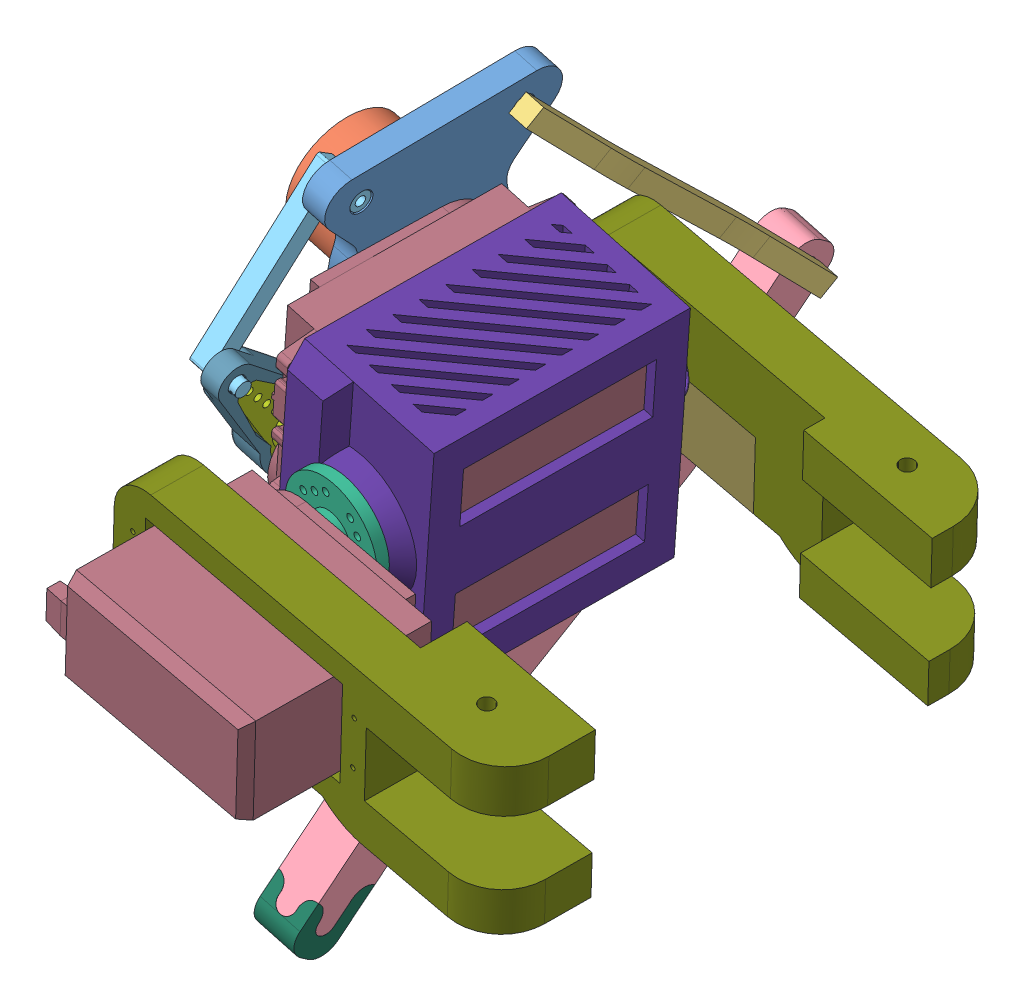
SolidWorks assembly Rear Reverse Robot Assembly, configuration Default. Lengths in mm.
30 component instances, 17 part files, 39 mates.
Components (placement in the parent):
- RearRotatingPiece-1: RearRotatingPiece [Default] at (10.5096 156.6748 85.525) x (-0.181401 -0.964552 0.191659) z (-0.041462 0.202221 0.978462) size (44.28 6 43.21)
- RearUpperLeg-1: RearUpperLeg [Default] at (2.9325 85.5783 8.4543) x (0.173114 0.681755 -0.710803) z (0.982535 -0.169547 0.076676) size (22 116.4 18)
- RearLongConnectingRod-1: RearLongConnectingRod [Default] at (-36.6414 185.2642 69.5457) x (-0.173068 -0.681269 0.71128) z (-0.068359 -0.712128 -0.698714) size (5 22 107.31)
- RearLowerLeg-1: RearLowerLeg [Default] at (-10.8789 13.8667 85.5543) x (0.037011 0.581891 0.812424) z (-0.982535 0.169547 -0.076676) size (20.21 126 9.59)
- RearShortConnectingRod-1: RearShortConnectingRod [Default] at (10.8355 144.2981 121.7991) x (0.184092 0.825622 -0.533346) z (0.982535 -0.169547 0.076676) size (37.08 4 13)
- Circle Rudder-1: Circle Rudder [默认] at (11.4281 139.3867 122.2016) x (0.455641 -0.889568 -0.032554) z (-0.885415 -0.449136 -0.119653) size (20.8 5.5 20.8)
- Double_Blade_Rudder-1: Double_Blade_Rudder [默认] at (-20.7962 133.019 101.8047) x (-0.170361 -0.653871 0.737177) z (0.07485 0.737365 0.671335) size (12.2 5.5 38)
- 688ZZ Bearing Assembly-1: 688ZZ Bearing Assembly [Default] at (17.0351 144.3872 61.4644) x (0.995768 -0.003841 0.091818) z (-0.091818 -0.083342 0.992282) size (17.99 17.98 5)
  - Outer Ring-1: Outer Ring [Default] at origin size (16 16 5)
  - Inner Ring-1: Inner Ring [Default] x (-0.241565 -0.970385 0) z (0 0 1) size (10.6 10.6 5)
  - Cage-1: Cage [Default] x (0.535517 0.844524 0) z (0 0 1) size (13.01 13.06 2.21)
  - 2mm Ball Bearing-1: 2mm Ball Bearing [Default] at (-5.0671 3.2131 0) x (0.050652 0.835774 0.546732) z (0.977207 -0.154478 0.145614) size (2 2 2)
  - 2mm Ball Bearing-2: 2mm Ball Bearing [Default] at (-5.988 -0.3789 0) x (-0.450278 0.705928 0.546732) z (0.881377 0.449412 0.145614) size (2 2 2)
  - 2mm Ball Bearing-3: 2mm Ball Bearing [Default] at (-4.6217 -3.8262 0) x (-0.779216 0.306441 0.546732) z (0.448891 0.881642 0.145614) size (2 2 2)
  - 2mm Ball Bearing-4: 2mm Ball Bearing [Default] at (-1.49 -5.812 0) x (-0.810521 -0.210096 0.546732) z (-0.155056 0.977115 0.145614) size (2 2 2)
  - 2mm Ball Bearing-5: 2mm Ball Bearing [Default] at (2.2108 -5.5778 0) x (-0.532234 -0.646383 0.546732) z (-0.699777 0.699363 0.145614) size (2 2 2)
  - 2mm Ball Bearing-6: 2mm Ball Bearing [Default] at (5.0671 -3.2131 0) x (-0.050652 -0.835774 0.546732) z (-0.977207 0.154478 0.145614) size (2 2 2)
  - 2mm Ball Bearing-7: 2mm Ball Bearing [Default] at (5.988 0.3789 0) x (0.450278 -0.705928 0.546732) z (-0.881377 -0.449412 0.145614) size (2 2 2)
  - 2mm Ball Bearing-8: 2mm Ball Bearing [Default] at (4.6217 3.8262 0) x (0.779216 -0.306441 0.546732) z (-0.448891 -0.881642 0.145614) size (2 2 2)
  - 2mm Ball Bearing-9: 2mm Ball Bearing [Default] at (1.49 5.812 0) x (0.810521 0.210096 0.546732) z (0.155056 -0.977115 0.145614) size (2 2 2)
  - 2mm Ball Bearing-10: 2mm Ball Bearing [Default] at (-2.2108 5.5778 0) x (0.532234 0.646383 0.546732) z (0.699777 -0.699363 0.145614) size (2 2 2)
- Lower Leg Mount-1: Lower Leg Mount [Default] at (-1.7272 146.59 62.4328) x (-0.988411 0.128599 -0.080659) z (0.091818 0.083342 -0.992282) size (41.75 15.4 10)
- MG996R-3: MG996R [Default] at (17.6577 134.1817 167.7413) x (0.988411 -0.128599 0.080659) z (0.120884 0.988188 0.094184) size (54.5 42.75 20)
- Circle Rudder-2: Circle Rudder [默认] at (-14.3485 160.9643 83.5851) x (-0.185428 -0.85768 0.479585) z (0.015549 0.485427 0.874139) size (20.8 5.5 20.8)
- MG996R-4: MG996R [Default] at (24.6112 126.1226 94.8455) x (0.091818 0.083342 -0.992282) z (0.161848 0.981992 0.097454) size (54.5 42.75 20)
- MG996R-5: MG996R [Default] at (28.967 152.5506 97.4682) x (-0.091818 -0.083342 0.992282) z (-0.161848 -0.981992 -0.097454) size (54.5 42.75 20)
- Servo Arm Mount-1: Servo Arm Mount [Default] at (-20.8945 133.036 101.7971) x (-0.170361 -0.653871 0.737177) z (-0.982535 0.169547 -0.076676) size (16.2 34.39 7.06)
- Foot Cap-1: Foot Cap [Default] at (-37.1895 24.1002 67.1144) x (0.037011 0.581891 0.812424) z (-0.982535 0.169547 -0.076676) size (10.5 14 9.53)
- Rear Reverse eg Mount-1: Rear Reverse eg Mount [Default] at (-93.0222 185.9824 -70.1903) x (0.988411 -0.128599 0.080659) z (-0.091818 -0.083342 0.992282) size (86 33.8 96.5)
- RearServoHousing-1: RearServoHousing [Default] at (-11.9904 86.4431 88.1259) x (0.091818 0.083342 -0.992282) z (-0.982535 0.169547 -0.076676) size (61.5 52 29.25)
Mates (geometry in assembly coordinates):
- Concentric12: concentric aligned: cylinder of Circle Rudder-2 through (-12.0887 160.5744 83.7615) axis (-0.982535 0.169547 -0.076676) radius 1.5; cylinder of MG996R-5 through (-9.1411 160.0657 83.9915) axis (-0.982535 0.169547 -0.076676) radius 1.5
- Coincident20: coincident anti-aligned: plane of Circle Rudder-2 through (-12.0887 160.5744 83.7615) normal (0.982535 -0.169547 0.076676); plane of MG996R-5 through (-12.0887 160.5744 83.7615) normal (-0.982535 0.169547 -0.076676)
- Coincident21: coincident anti-aligned: plane of RearUpperLeg-1 through (-14.3485 160.9643 83.5851) normal (0.982535 -0.169547 0.076676); plane of Circle Rudder-2 through (-14.3485 160.9643 83.5851) normal (-0.982535 0.169547 -0.076676)
- Concentric13: concentric anti-aligned: cylinder of RearUpperLeg-1 through (-23.1914 162.4902 82.8951) axis (0.982535 -0.169547 0.076676) radius 1.7; cylinder of Circle Rudder-2 through (-12.0887 160.5744 83.7615) axis (-0.982535 0.169547 -0.076676) radius 1.5
- Concentric14: concentric anti-aligned: cylinder of RearRotatingPiece-1 through (-11.1062 160.4048 83.8382) axis (0.982535 -0.169547 0.076676) radius 4.5; cylinder of Circle Rudder-2 through (-8.9446 160.0318 84.0069) axis (-0.982535 0.169547 -0.076676) radius 4.4
- Coincident22: coincident anti-aligned: plane of RearRotatingPiece-1 through (-9.1411 160.0657 83.9915) normal (0.982535 -0.169547 0.076676); plane of MG996R-5 through (-9.1411 160.0657 83.9915) normal (-0.982535 0.169547 -0.076676)
- Concentric16: concentric aligned: cylinder of Double_Blade_Rudder-1 through (-18.5364 132.6291 101.9811) axis (-0.982535 0.169547 -0.076676) radius 1.5; cylinder of MG996R-4 through (-15.3923 132.0865 102.2264) axis (-0.982535 0.169547 -0.076676) radius 1.5
- Coincident24: coincident anti-aligned: plane of Double_Blade_Rudder-1 through (-15.3923 132.0865 102.2264) normal (0.982535 -0.169547 0.076676); plane of MG996R-4 through (-15.3923 132.0865 102.2264) normal (-0.982535 0.169547 -0.076676)
- Coincident25: coincident anti-aligned: plane of Double_Blade_Rudder-1 through (-20.7962 133.019 101.8047) normal (-0.982535 0.169547 -0.076676); plane of Servo Arm Mount-1 through (-20.7962 133.019 101.8047) normal (0.982535 -0.169547 0.076676)
- Concentric17: concentric aligned: cylinder of Double_Blade_Rudder-1 through (-18.5364 132.6291 101.9811) axis (-0.982535 0.169547 -0.076676) radius 1.5; cylinder of Servo Arm Mount-1 through (-20.7962 133.019 101.8047) axis (-0.982535 0.169547 -0.076676) radius 1.6
- Concentric18: concentric anti-aligned: cylinder of RearRotatingPiece-1 through (-12.4518 177.2224 99.1423) axis (0.982535 -0.169547 0.076676) radius 2.2; cylinder of RearShortConnectingRod-1 through (-7.7356 176.4086 99.5103) axis (-0.982535 0.169547 -0.076676) radius 2
- Concentric19: concentric aligned: cylinder of RearShortConnectingRod-1 through (-13.899 148.7667 117.3667) axis (-0.982535 0.169547 -0.076676) radius 1.5; cylinder of Servo Arm Mount-1 through (-15.2745 149.0041 117.2594) axis (-0.982535 0.169547 -0.076676) radius 1.7
- Coincident27: coincident anti-aligned: plane of RearShortConnectingRod-1 through (-19.4266 149.5201 119.4375) normal (0.982535 -0.169547 0.076676); plane of Servo Arm Mount-1 through (-20.8945 133.036 101.7971) normal (-0.982535 0.169547 -0.076676)
- Concentric23: concentric aligned: cylinder of RearUpperLeg-1 through (-17.2701 88.8319 13.689) axis (-0.982535 0.169547 -0.076676) radius 2.1; cylinder of RearLowerLeg-1 through (-21.6915 89.5949 13.344) axis (-0.982535 0.169547 -0.076676) radius 2
- Distance3: distance = 0.5 mm anti-aligned: plane of RearLowerLeg-1 through (-48.2153 20.3095 82.6406) normal (-0.982535 0.169547 -0.076676); plane of RearUpperLeg-1 through (-33.2435 80.4348 17.2202) normal (0.982535 -0.169547 0.076676)
- Concentric26: concentric aligned: cylinder of RearLowerLeg-1 through (-41.8818 25.7841 72.2765) axis (-0.037011 -0.581891 -0.812424) radius 2; cylinder of Foot Cap-1 through (-41.6967 28.6936 76.3386) axis (-0.037011 -0.581891 -0.812424) radius 2
- Concentric27: concentric aligned: cylinder of RearLowerLeg-1 through (-47.3061 22.1724 75.1105) axis (0.982535 -0.169547 0.076676) radius 2; cylinder of Foot Cap-1 through (-47.3061 22.1724 75.1105) axis (0.982535 -0.169547 0.076676) radius 2
- Concentric28: concentric aligned: cylinder of MG996R-3 through (-5.1273 134.9523 138.2357) axis (0.091818 0.083342 -0.992282) radius 1.7678; circle of Rear Reverse eg Mount-1
- Parallel1: parallel aligned: plane of MG996R-3 through (2.1338 149.6472 131.5757) normal (0.120884 0.988188 0.094184); plane of Rear Reverse eg Mount-1 through (40.0248 122.8761 151.4782) normal (0.120884 0.988188 0.094184)
- Coincident33: coincident anti-aligned: plane of MG996R-3 through (-5.1273 134.9523 138.2357) normal (-0.091818 -0.083342 0.992282); plane of Rear Reverse eg Mount-1 through (-19.2198 54.6372 130.186) normal (0.091818 0.083342 -0.992282)
- Concentric29: concentric aligned: cylinder of Circle Rudder-1 through (11.2169 139.1951 124.4839) axis (0.091818 0.083342 -0.992282) radius 1.5; cylinder of MG996R-3 through (10.9414 138.945 127.4607) axis (0.091818 0.083342 -0.992282) radius 1.5
- Coincident34: coincident anti-aligned: plane of Circle Rudder-1 through (11.2169 139.1951 124.4839) normal (-0.091818 -0.083342 0.992282); plane of MG996R-3 through (11.2169 139.1951 124.4839) normal (0.091818 0.083342 -0.992282)
- Concentric30: concentric aligned: cylinder of 688ZZ Bearing Assembly-1/Outer Ring-1 through (16.4148 143.8241 68.1677) axis (-0.091818 -0.083342 0.992282) radius 8; cylinder of Rear Reverse eg Mount-1 through (17.7237 145.0122 54.0223) axis (-0.091818 -0.083342 0.992282) radius 8
- Coincident35: coincident aligned: plane of 688ZZ Bearing Assembly-1/Outer Ring-1 through (16.7787 151.1544 64.5285) normal (-0.091818 -0.083342 0.992282); plane of Rear Reverse eg Mount-1 through (-12.1957 61.0129 54.2764) normal (-0.091818 -0.083342 0.992282)
- Coincident36: coincident anti-aligned: plane of Lower Leg Mount-1 through (25.631 143.9834 54.6676) normal (0.120884 0.988188 0.094184); plane of Rear Reverse eg Mount-1 through (24.7128 143.15 64.5904) normal (-0.120884 -0.988188 -0.094184)
- Coincident37: coincident anti-aligned: plane of Lower Leg Mount-1 through (40.4572 142.0545 55.8774) normal (0.988411 -0.128599 0.080659); plane of Rear Reverse eg Mount-1 through (39.539 141.221 65.8003) normal (-0.988411 0.128599 -0.080659)
- Coincident38: coincident aligned: plane of Lower Leg Mount-1 through (17.7237 145.0122 54.0223) normal (0.091818 0.083342 -0.992282); plane of Rear Reverse eg Mount-1 through (86.056 151.5821 60.897) normal (0.091818 0.083342 -0.992282)
- Concentric32: concentric aligned: cylinder of 688ZZ Bearing Assembly-1/Inner Ring-1 through (16.4148 143.8241 68.1677) axis (-0.091818 -0.083342 0.992282) radius 4; cylinder of RearServoHousing-1 through (17.0626 144.4122 61.1667) axis (-0.091818 -0.083342 0.992282) radius 4
- Coincident40: coincident anti-aligned: plane of Circle Rudder-1 through (11.4281 139.3867 122.2016) normal (0.091818 0.083342 -0.992282); plane of RearServoHousing-1 through (96.195 111.5281 127.7054) normal (-0.091818 -0.083342 0.992282)
- Concentric33: concentric anti-aligned: cylinder of MG996R-5 through (0.6697 159.7731 120.6509) axis (-0.982535 0.169547 -0.076676) radius 1.7678; circle of RearServoHousing-1
- Parallel2: parallel anti-aligned: plane of MG996R-5 through (-2.6809 170.1195 75.6079) normal (0.161848 0.981992 0.097454); plane of RearServoHousing-1 through (104.5236 149.1508 104.1741) normal (-0.161848 -0.981992 -0.097454)
- Coincident42: coincident anti-aligned: plane of MG996R-5 through (28.967 152.5506 97.4682) normal (0.982535 -0.169547 0.076676); plane of RearServoHousing-1 through (24.685 126.5707 94.8899) normal (-0.982535 0.169547 -0.076676)
- Parallel3: parallel anti-aligned: plane of MG996R-4 through (-10.7553 140.3162 113.1726) normal (0.161848 0.981992 0.097454); plane of RearServoHousing-1 through (100.3155 123.6191 101.6403) normal (-0.161848 -0.981992 -0.097454)
- Concentric34: concentric anti-aligned: cylinder of MG996R-4 through (-5.2306 123.9733 117.0981) axis (-0.982535 0.169547 -0.076676) radius 1.7678; circle of RearServoHousing-1
- Coincident45: coincident anti-aligned: plane of MG996R-4 through (24.6112 126.1226 94.8455) normal (0.982535 -0.169547 0.076676); plane of RearServoHousing-1 through (24.685 126.5707 94.8899) normal (-0.982535 0.169547 -0.076676)
- Concentric35: concentric anti-aligned: cylinder of RearLongConnectingRod-1 through (-25.1893 110.8701 -1.7349) axis (0.982535 -0.169547 0.076676) radius 2; cylinder of RearLowerLeg-1 through (-17.1325 109.4798 -1.1061) axis (-0.982535 0.169547 -0.076676) radius 2.1
- Concentric36: concentric aligned: cylinder of RearRotatingPiece-1 through (-9.5106 180.5569 68.8266) axis (0.982535 -0.169547 0.076676) radius 2.2; cylinder of RearLongConnectingRod-1 through (-10.6896 180.7604 68.7346) axis (0.982535 -0.169547 0.076676) radius 2
- Coincident47: coincident anti-aligned: plane of RearRotatingPiece-1 through (-9.1411 160.0657 83.9915) normal (0.982535 -0.169547 0.076676); plane of RearLongConnectingRod-1 through (-4.8073 179.7709 72.03) normal (-0.982535 0.169547 -0.076676)
- Concentric37: concentric aligned: cylinder of Double_Blade_Rudder-1 through (-17.5633 142.2148 110.7084) axis (-0.982535 0.169547 -0.076676) radius 0.75; cylinder of Servo Arm Mount-1 through (-19.8231 142.6048 110.5321) axis (-0.982535 0.169547 -0.076676) radius 0.75
